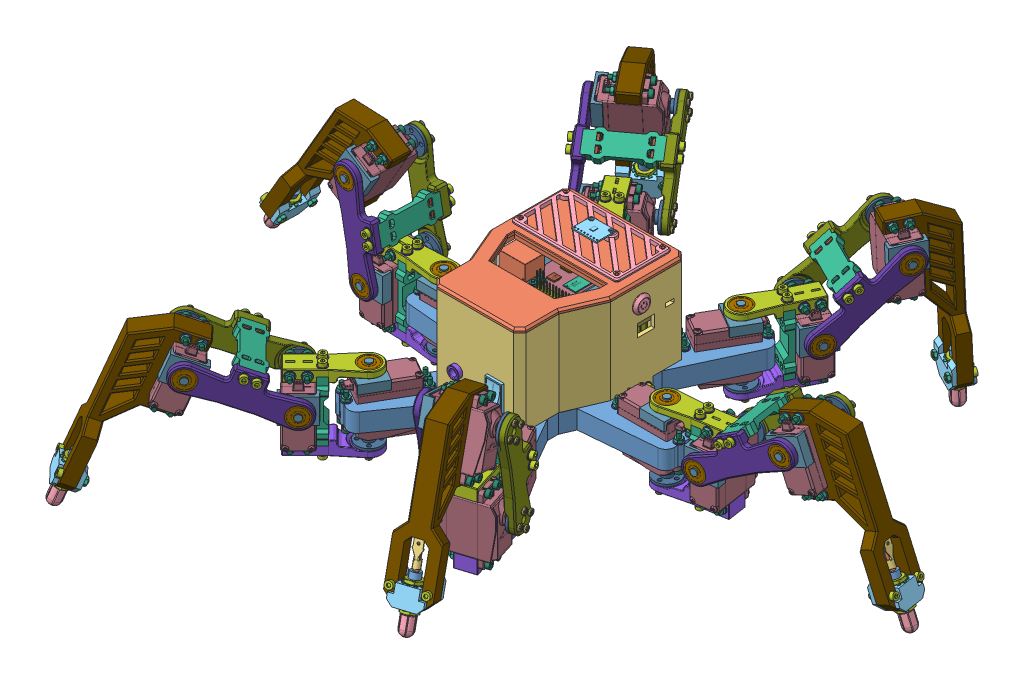
SolidWorks assembly HEXUMI_DSSERVO, configuration Default. Lengths in mm. (continued)
Components (placement in the parent): (continued)
- LEG_L-2: LEG_L [Default] at (-76.6324 -8.25 141.7647) x (0.700512 0 0.713641) z (0.713641 0 -0.700512) size (67.5 173.11 232.67) (flexible) (continued)
  - M3_SERVO_HORN_BOLT-12: M3_SERVO_HORN_BOLT [Default] at (-34.5 -12.4934 -16.7216) x (0 0.672311 -0.740269) z (0 -0.740269 -0.672311) size (4.8 7 4.8)
  - M3_SERVO_HORN_BOLT-13: M3_SERVO_HORN_BOLT [Default] at (-29.5 -35.3838 -75.416) x (0 0.520293 -0.853988) z (0 -0.853988 -0.520293) size (4.8 7 4.8)
  - M3_SERVO_HORN_BOLT-14: M3_SERVO_HORN_BOLT [Default] at (-29.5 -9.95 -10.2) x (0 0.520293 -0.853988) z (0 -0.853988 -0.520293) size (4.8 7 4.8)
  - M3_STEEL_HEX_BOLT_16MM-6: M3_STEEL_HEX_BOLT_16MM [Default] at (-36 -37.6293 -41.2662) x (0 -0.255744 -0.966745) z (0 -0.966745 0.255744) size (5.68 19 5.68)
  - M3_STEEL_HEX_BOLT_16MM-7: M3_STEEL_HEX_BOLT_16MM [Default] at (31.5 -37.6293 -41.2662) x (0 0.850981 0.525196) z (0 -0.525196 0.850981) size (5.68 19 5.68)
  - M3_STEEL_HEX_BOLT_16MM-8: M3_STEEL_HEX_BOLT_16MM [Default] at (-36 -34.7226 -33.8129) x (0 -0.563912 -0.825835) z (0 -0.825835 0.563912) size (5.68 19 5.68)
  - M3_WASHER-10: M3_WASHER [Default] at (28.5 -37.6293 -41.2662) x (0 0.320127 0.947375) z (0 -0.947375 0.320127) size (7 0.5 7)
  - M3_WASHER-11: M3_WASHER [Default] at (-32.5 -37.6293 -41.2662) x (0 0.222061 0.975033) z (0 -0.975033 0.222061) size (7 0.5 7)
  - M3_WASHER-12: M3_WASHER [Default] at (-32.5 -34.7226 -33.8129) x (0 0.409501 0.91231) z (0 -0.91231 0.409501) size (7 0.5 7)
  - M3_SQUARE_NUT-10: M3_SQUARE_NUT [Default] at (14.7 -37.6293 -41.2662) x (0 0.36334 0.931657) z (0 -0.931657 0.36334) size (5.3 1.7 5.3)
  - M3_SQUARE_NUT-11: M3_SQUARE_NUT [Default] at (14.7 -34.7226 -33.8129) x (0 0.36334 0.931657) z (0 -0.931657 0.36334) size (5.3 1.7 5.3)
  - M3_SQUARE_NUT-12: M3_SQUARE_NUT [Default] at (-17.5 -37.6293 -41.2662) x (0 0.36334 0.931657) z (0 -0.931657 0.36334) size (5.3 1.7 5.3)
  - SERVO_ASM-3: SERVO_ASM [Default] at (-25.8 -35.3838 -75.416) x (0 0.932062 -0.3623) z (-1 0 0) size (87.25 24.4 54.8)
    - SW2020 DS3225MG Servo 25Kg 4.8-6.8V-2: SW2020 DS3225MG Servo 25Kg 4.8-6.8V [Default] at origin size (54.3 20.4 45.91)
    - SERVO_CLIP-1: SERVO_CLIP [Default] at (0 0 -45.6) x (-1 0 0) z (0 0 -1) size (20 24.4 14.2)
  - M3_STEEL_HEX_BOLT-6: M3_STEEL_HEX_BOLT [Default] at (-14.2 -47.3668 -65.3936) x (0 -0.933228 -0.359286) z (0 -0.359286 0.933228) size (5.68 28 5.68)
  - M3_STEEL_HEX_BOLT-7: M3_STEEL_HEX_BOLT [Default] at (-14.2 -1.1366 -83.3637) x (0 -0.933228 -0.359286) z (0 -0.359286 0.933228) size (5.68 28 5.68)
  - M3_STEEL_HEX_BOLT-8: M3_STEEL_HEX_BOLT [Default] at (-14.2 -4.7596 -92.6843) x (0 -0.933228 -0.359286) z (0 -0.359286 0.933228) size (5.68 28 5.68)
  - M3_WASHER-13: M3_WASHER [Default] at (8.5 -50.9898 -74.7142) x (0 -0.744989 0.667077) z (0 -0.667077 -0.744989) size (7 0.5 7)
  - M3_WASHER-14: M3_WASHER [Default] at (8.5 -1.1366 -83.3637) x (0 0.510645 0.859791) z (0 -0.859791 0.510645) size (7 0.5 7)
  - M3_WASHER-15: M3_WASHER [Default] at (8.5 -47.3668 -65.3936) x (0 -0.855136 -0.518404) z (0 0.518404 -0.855136) size (7 0.5 7)
  - M3_HEX_NUT-9: M3_HEX_NUT [Default] at (8.5 -50.9898 -74.7142) x (0 -0.742673 0.669654) z (0 0.669654 0.742673) size (6.98 2.4 5.5)
  - M3_HEX_NUT-10: M3_HEX_NUT [Default] at (8.5 -47.3668 -65.3936) x (0 -0.972142 0.234393) z (0 0.234393 0.972142) size (6.98 2.4 5.5)
  - M3_HEX_NUT-11: M3_HEX_NUT [Default] at (8.5 -4.7596 -92.6843) x (0 -0.862059 0.506808) z (0 0.506808 0.862059) size (6.98 2.4 5.5)
  - M3_WASHER-17: M3_WASHER [Default] at (8.5 -4.7596 -92.6843) x (0 -0.944852 -0.327497) z (0 0.327497 -0.944852) size (7 0.5 7)
  - M3_SERVO_HORN_BOLT-15: M3_SERVO_HORN_BOLT [Default] at (0 28.25 30) x (0.299137 0 -0.95421) z (-0.95421 0 -0.299137) size (4.8 7 4.8)
  - TIBIA_V2_ASM-1: TIBIA_V2_ASM [Default] at (0 -35.2725 -75.4056) x (-1 0 0) z (0 -0.932062 0.3623) size (32.11 50.6 145.7)
    - TIBIA_V2-1: TIBIA_V2 [Default] at origin size (32 47.6 127.94)
    - LIMIT_SWITCH-1: LIMIT_SWITCH [Default] at (0 32.3524 -111.7407) x (-0.992713 0.1205 0) z (0.1205 0.992713 0) size (13.8 62.3 13.8) (flexible)
      - LIMIT_SWITCH_SLEEVE-1: LIMIT_SWITCH_SLEEVE [Default] at origin size (7.7 25.25 7.7)
      - LIMIT_SWITCH_SHAFT-1: LIMIT_SWITCH_SHAFT [Default] at (0 5.5422 0) x (-0.210419 0 -0.977611) z (0.977611 0 -0.210419) size (5 52 5)
      - LIMIT_SWITCH_LIMITER-1: LIMIT_SWITCH_LIMITER [Default] at (0 26.0422 0) x (-0.600712 0 -0.799465) z (0.799465 0 -0.600712) size (6.64 21.41 7.08)
      - RUBBER_CAP-1: RUBBER_CAP [Default] at (0 -9.9578 0) x (0.575853 0 -0.817553) z (0.817553 0 0.575853) size (10 14 10)
    - FOOT_HOLD-1: FOOT_HOLD [Default] at (0 32.3524 -108.9407) x (1 0 0) z (0 -1 0) size (32 22 16)
    - LIMIT_SWITCH_WASHER-1: LIMIT_SWITCH_WASHER [Default] at (0 32.3524 -93.5407) x (0.999093 -0.042592 0) z (0.042592 0.999093 0) size (14.82 0.4 15)
    - LIMIT_SWITCH_WASHER-2: LIMIT_SWITCH_WASHER [Default] at (0 32.3524 -108.9407) x (0.999093 -0.042592 0) z (0.042592 0.999093 0) size (14.82 0.4 15)
    - LIMIT_SWITCH_NUT-1: LIMIT_SWITCH_NUT [Default] at (0 32.3524 -92.3407) x (0.997292 -0.073548 0) z (0.073548 0.997292 0) size (13.86 2.4 12)
    - LIMIT_SWITCH_NUT-2: LIMIT_SWITCH_NUT [Default] at (0 32.3524 -110.5407) x (0.999648 -0.026514 0) z (0.026514 0.999648 0) size (13.86 2.4 12)
    - M3_HEX_NUT-1: M3_HEX_NUT [Default] at (-12 21.9524 -96.9407) x (-0.996596 0 -0.082443) z (0.082443 0 -0.996596) size (6.98 2.4 5.5)
    - M3_HEX_NUT-2: M3_HEX_NUT [Default] at (12 21.9524 -96.9407) x (-0.491735 0 -0.870745) z (0.870745 0 -0.491735) size (6.98 2.4 5.5)
    - M3_STEEL_HEX_BOLT_16MM-1: M3_STEEL_HEX_BOLT_16MM [Default] at (-12 40.3524 -96.9407) x (-0.809803 0 -0.586702) z (-0.586702 0 0.809803) size (5.68 19 5.68)
    - M3_STEEL_HEX_BOLT_16MM-2: M3_STEEL_HEX_BOLT_16MM [Default] at (12 40.3524 -96.9407) x (-0.933551 0 -0.358443) z (-0.358443 0 0.933551) size (5.68 19 5.68)
- LEG_L-3: LEG_L [Default] at (-120.0853 -8.25 24.3604) x (-0.031319 0 0.999509) z (0.999509 0 0.031319) size (67.5 177.61 179.91) (flexible)
  - LINK-1: LINK [Default] at origin size (20 48.5 7)
  - COXA_BEARING-1: COXA_BEARING [Default] at (0 -29.25 30) size (20 9.2 60)
  - COXA_SERVO-1: COXA_SERVO [Default] at (0 31.25 30) x (-1 0 0) z (0 0 1) size (20 11.2 60)
  - BEARING-1: BEARING [Default] at (0 -24.25 30) x (-0.081882 0 0.996642) z (0 -1 0) size (16 16 5)
  - HORN-1: HORN [Default] at (0 26.25 30) x (0 0 -1) z (0 -1 0) size (20 20 4.6)
  - M3_SQUARE_NUT-1: M3_SQUARE_NUT [Default] at (-4 16.25 3.5) x (0.988939 0 -0.14832) z (0.14832 0 0.988939) size (5.3 1.7 5.3)
  - M3_STEEL_HEX_BOLT_16MM-1: M3_STEEL_HEX_BOLT_16MM [Default] at (4 34.75 3.5) x (-0.949613 0 0.313425) z (0.313425 0 0.949613) size (5.68 19 5.68)
  - M3_WASHER-1: M3_WASHER [Default] at (4 31.25 3.5) x (0.934731 0 0.355356) z (-0.355356 0 0.934731) size (7 0.5 7)
  - M3_SERVO_HORN_BOLT-1: M3_SERVO_HORN_BOLT [Default] at (-7 33.25 30) x (-0.685901 0 -0.727695) z (-0.727695 0 0.685901) size (4.8 7 4.8)
  - M3_SERVO_HORN_BOLT-2: M3_SERVO_HORN_BOLT [Default] at (7 33.25 30) x (-0.685901 0 -0.727695) z (-0.727695 0 0.685901) size (4.8 7 4.8)
  - M3_SERVO_HORN_BOLT-3: M3_SERVO_HORN_BOLT [Default] at (0 33.25 37) x (-0.685901 0 -0.727695) z (-0.727695 0 0.685901) size (4.8 7 4.8)
  - M3_SERVO_HORN_BOLT-4: M3_SERVO_HORN_BOLT [Default] at (0 33.25 23) x (-0.685901 0 -0.727695) z (-0.727695 0 0.685901) size (4.8 7 4.8)
  - M3_SQUARE_NUT-2: M3_SQUARE_NUT [Default] at (4 16.25 3.5) x (0.988939 0 -0.14832) z (0.14832 0 0.988939) size (5.3 1.7 5.3)
  - M3_SQUARE_NUT-3: M3_SQUARE_NUT [Default] at (-4 -15.95 3.5) x (0.988939 0 -0.14832) z (0.14832 0 0.988939) size (5.3 1.7 5.3)
  - M3_SQUARE_NUT-4: M3_SQUARE_NUT [Default] at (4 -15.95 3.5) x (0.988939 0 -0.14832) z (0.14832 0 0.988939) size (5.3 1.7 5.3)
  - M3_STEEL_HEX_BOLT_16MM-2: M3_STEEL_HEX_BOLT_16MM [Default] at (-4 -32.75 3.5) x (0.988939 0 -0.14832) z (0.14832 0 0.988939) size (5.68 19 5.68)
  - M3_STEEL_HEX_BOLT_16MM-3: M3_STEEL_HEX_BOLT_16MM [Default] at (4 -32.75 3.5) x (0.988939 0 -0.14832) z (0.14832 0 0.988939) size (5.68 19 5.68)
  - M3_STEEL_HEX_BOLT_16MM-4: M3_STEEL_HEX_BOLT_16MM [Default] at (-4 34.75 3.5) x (-0.85786 0 0.513883) z (0.513883 0 0.85786) size (5.68 19 5.68)
  - M3_WASHER-2: M3_WASHER [Default] at (4 -29.75 3.5) x (0.985952 0 -0.167027) z (0.167027 0 0.985952) size (7 0.5 7)
  - M3_WASHER-3: M3_WASHER [Default] at (-4 -29.75 3.5) x (0.922631 0 -0.385683) z (0.385683 0 0.922631) size (7 0.5 7)
  - M3_WASHER-4: M3_WASHER [Default] at (-4 31.25 3.5) x (0.993655 0 0.112474) z (-0.112474 0 0.993655) size (7 0.5 7)
  - SERVO_ASM-1: SERVO_ASM [Default] at (-25.8 -9.95 -10.2) x (0 1 0) z (-1 0 0) size (87.25 24.4 54.8)
    - SW2020 DS3225MG Servo 25Kg 4.8-6.8V-2: SW2020 DS3225MG Servo 25Kg 4.8-6.8V [Default] at origin size (54.3 20.4 45.91)
    - SERVO_CLIP-1: SERVO_CLIP [Default] at (0 0 -45.6) x (-1 0 0) z (0 0 -1) size (20 24.4 14.2)
  - SERVO_ASM-2: SERVO_ASM [Default] at (0 24.55 30) x (-0.031319 0 0.999509) z (0 1 0) size (87.25 24.4 54.8)
    - SW2020 DS3225MG Servo 25Kg 4.8-6.8V-2: SW2020 DS3225MG Servo 25Kg 4.8-6.8V [Default] at origin size (54.3 20.4 45.91)
    - SERVO_CLIP-1: SERVO_CLIP [Default] at (0 0 -45.6) x (-1 0 0) z (0 0 -1) size (20 24.4 14.2)
  - M3_HEX_NUT-1: M3_HEX_NUT [Default] at (10.4 -24.75 -15.2) x (0 0.554401 -0.83225) z (0 0.83225 0.554401) size (6.98 2.4 5.5)
  - M3_SQUARE_NUT-5: M3_SQUARE_NUT [Default] at (0.85 24.85 -15.2) x (0 0 -1) z (0 1 0) size (5.3 1.7 5.3)
  - M3_STEEL_HEX_BOLT-1: M3_STEEL_HEX_BOLT [Default] at (-14.2 -24.75 -5.2) x (0 -0.390994 0.920393) z (0 0.920393 0.390994) size (5.68 28 5.68)
  - M3_WASHER-5: M3_WASHER [Default] at (8 -24.75 -5.2) x (0 -0.313666 0.949533) z (0 0.949533 0.313666) size (7 0.5 7)
  - M3_WASHER-6: M3_WASHER [Default] at (8 -24.75 -15.2) x (0 -0.313666 0.949533) z (0 0.949533 0.313666) size (7 0.5 7)
  - M3_WASHER-7: M3_WASHER [Default] at (8 24.85 -15.2) x (0 -0.313666 0.949533) z (0 0.949533 0.313666) size (7 0.5 7)
  - M3_WASHER-8: M3_WASHER [Default] at (8 24.85 -5.2) x (0 -0.313666 0.949533) z (0 0.949533 0.313666) size (7 0.5 7)
  - M3_STEEL_HEX_BOLT-2: M3_STEEL_HEX_BOLT [Default] at (-14.2 24.85 -15.2) x (0 -0.835258 0.549858) z (0 0.549858 0.835258) size (5.68 28 5.68)
  - M3_STEEL_HEX_BOLT-3: M3_STEEL_HEX_BOLT [Default] at (-14.2 -24.75 -15.2) x (0 0.230066 0.973175) z (0 0.973175 -0.230066) size (5.68 28 5.68)
  - M3_STEEL_HEX_BOLT-4: M3_STEEL_HEX_BOLT [Default] at (-14.2 24.85 -5.2) x (0 -0.984641 0.17459) z (0 0.17459 0.984641) size (5.68 28 5.68)
  - M3_SQUARE_NUT-6: M3_SQUARE_NUT [Default] at (0.85 -24.75 -5.2) x (0 1 0) z (0 0 1) size (5.3 1.7 5.3)
  - M3_SQUARE_NUT-7: M3_SQUARE_NUT [Default] at (0.85 -24.75 -15.2) x (0 1 0) z (0 0 1) size (5.3 1.7 5.3)
  - M3_SQUARE_NUT-8: M3_SQUARE_NUT [Default] at (0.85 24.85 -5.2) x (0 0 -1) z (0 1 0) size (5.3 1.7 5.3)
  - M3_HEX_NUT-2: M3_HEX_NUT [Default] at (10.4 -24.75 -5.2) x (0 0.450627 -0.892712) z (0 0.892712 0.450627) size (6.98 2.4 5.5)
  - M3_HEX_NUT-3: M3_HEX_NUT [Default] at (10.9 24.85 -5.2) x (0 0.387589 -0.921832) z (0 0.921832 0.387589) size (6.98 2.4 5.5)
  - M3_HEX_NUT-4: M3_HEX_NUT [Default] at (10.9 24.85 -15.2) x (0 0.281781 -0.959479) z (0 0.959479 0.281781) size (6.98 2.4 5.5)
  - FEMUR_SERVO-1: FEMUR_SERVO [Default] at (-32.5 -78.7023 -23.3578) x (1 0 0) z (0 -0.982175 -0.187968) size (10 28 90)
  - FEMUR_BEARING-1: FEMUR_BEARING [Default] at (28 -9.95 -10.2) x (-1 0 0) z (0 0.982175 0.187968) size (8 28 90)
  - LINK-2: LINK [Default] at (-1.25 -47.7096 0.9003) x (0 -0.982175 -0.187968) z (0 0.187968 -0.982175) size (20 48.5 7)
  - BEARING-2: BEARING [Default] at (28 -9.95 -10.2) x (0 0.418384 0.90827) z (-1 0 0) size (16 16 5)
  - HORN-2: HORN [Default] at (-27.5 -9.95 -10.2) x (0 -0.187968 0.982175) z (1 0 0) size (20 20 4.6)
  - BEARING-3: BEARING [Default] at (28 -78.7023 -23.3578) x (0 0.417885 0.9085) z (-1 0 0) size (16 16 5)
  - HORN-3: HORN [Default] at (-27.5 -78.7023 -23.3578) x (0 0.982175 0.187968) z (1 0 0) size (20 20 4.6)
  - M3_HEX_NUT-5: M3_HEX_NUT [Default] at (8.5 -46.1809 -36.7145) x (0 -0.996607 0.082307) z (0 0.082307 0.996607) size (6.98 2.4 5.5)
  - M3_SERVO_HORN_BOLT-5: M3_SERVO_HORN_BOLT [Default] at (-34.5 -11.2658 -3.3248) x (0 0.998165 -0.060547) z (0 -0.060547 -0.998165) size (4.8 7 4.8)
  - M3_SQUARE_NUT-9: M3_SQUARE_NUT [Default] at (-17.5 -43.123 -1.7855) x (0 0.982175 0.187968) z (0 -0.187968 0.982175) size (5.3 1.7 5.3)
  - M3_STEEL_HEX_BOLT-5: M3_STEEL_HEX_BOLT [Default] at (-14.2 -93.9918 -20.1531) x (0 -0.933228 -0.359286) z (0 -0.359286 0.933228) size (5.68 28 5.68)
  - M3_STEEL_HEX_BOLT_16MM-5: M3_STEEL_HEX_BOLT_16MM [Default] at (31.5 -43.123 -1.7855) x (0 0.963892 0.266294) z (0 -0.266294 0.963892) size (5.68 19 5.68)
  - M3_WASHER-9: M3_WASHER [Default] at (28.5 -43.123 -1.7855) x (0 0.36047 0.932771) z (0 -0.932771 0.36047) size (7 0.5 7)
  - M3_SERVO_HORN_BOLT-6: M3_SERVO_HORN_BOLT [Default] at (-34.5 -8.6342 -17.0752) x (0 0.373361 -0.927686) z (0 -0.927686 -0.373361) size (4.8 7 4.8)
  - M3_SERVO_HORN_BOLT-7: M3_SERVO_HORN_BOLT [Default] at (-34.5 -71.827 -22.042) x (0 0.325507 -0.94554) z (0 -0.94554 -0.325507) size (4.8 7 4.8)
  - M3_SERVO_HORN_BOLT-8: M3_SERVO_HORN_BOLT [Default] at (-34.5 -77.3865 -30.233) x (0 0.184546 -0.982824) z (0 -0.982824 -0.184546) size (4.8 7 4.8)
  - M3_SERVO_HORN_BOLT-9: M3_SERVO_HORN_BOLT [Default] at (-34.5 -80.018 -16.4825) x (0 0.681327 -0.731979) z (0 -0.731979 -0.681327) size (4.8 7 4.8)
  - M3_SERVO_HORN_BOLT-10: M3_SERVO_HORN_BOLT [Default] at (-34.5 -85.5775 -24.6735) x (0 0.520293 -0.853988) z (0 -0.853988 -0.520293) size (4.8 7 4.8)
  - M3_SERVO_HORN_BOLT-11: M3_SERVO_HORN_BOLT [Default] at (-34.5 -3.0748 -8.8842) x (0 -0.171182 -0.985239) z (0 -0.985239 0.171182) size (4.8 7 4.8)
  - M3_SERVO_HORN_BOLT-12: M3_SERVO_HORN_BOLT [Default] at (-34.5 -16.8252 -11.5158) x (0 0.672311 -0.740269) z (0 -0.740269 -0.672311) size (4.8 7 4.8)
  - M3_SERVO_HORN_BOLT-13: M3_SERVO_HORN_BOLT [Default] at (-29.5 -78.7023 -23.3578) x (0 0.520293 -0.853988) z (0 -0.853988 -0.520293) size (4.8 7 4.8)
  - M3_SERVO_HORN_BOLT-14: M3_SERVO_HORN_BOLT [Default] at (-29.5 -9.95 -10.2) x (0 0.520293 -0.853988) z (0 -0.853988 -0.520293) size (4.8 7 4.8)
  - M3_STEEL_HEX_BOLT_16MM-6: M3_STEEL_HEX_BOLT_16MM [Default] at (-36 -50.9804 -3.2892) x (0 -0.255744 -0.966745) z (0 -0.966745 0.255744) size (5.68 19 5.68)
  - M3_STEEL_HEX_BOLT_16MM-7: M3_STEEL_HEX_BOLT_16MM [Default] at (31.5 -50.9804 -3.2892) x (0 0.850981 0.525196) z (0 -0.525196 0.850981) size (5.68 19 5.68)
  - M3_STEEL_HEX_BOLT_16MM-8: M3_STEEL_HEX_BOLT_16MM [Default] at (-36 -43.123 -1.7855) x (0 -0.563912 -0.825835) z (0 -0.825835 0.563912) size (5.68 19 5.68)
  - M3_WASHER-10: M3_WASHER [Default] at (28.5 -50.9804 -3.2892) x (0 0.320127 0.947375) z (0 -0.947375 0.320127) size (7 0.5 7)
  - M3_WASHER-11: M3_WASHER [Default] at (-32.5 -50.9804 -3.2892) x (0 0.222061 0.975033) z (0 -0.975033 0.222061) size (7 0.5 7)
  - M3_WASHER-12: M3_WASHER [Default] at (-32.5 -43.123 -1.7855) x (0 0.409501 0.91231) z (0 -0.91231 0.409501) size (7 0.5 7)
  - M3_SQUARE_NUT-10: M3_SQUARE_NUT [Default] at (14.7 -50.9804 -3.2892) x (0 0.982175 0.187968) z (0 -0.187968 0.982175) size (5.3 1.7 5.3)
  - M3_SQUARE_NUT-11: M3_SQUARE_NUT [Default] at (14.7 -43.123 -1.7855) x (0 0.982175 0.187968) z (0 -0.187968 0.982175) size (5.3 1.7 5.3)
  - M3_SQUARE_NUT-12: M3_SQUARE_NUT [Default] at (-17.5 -50.9804 -3.2892) x (0 0.982175 0.187968) z (0 -0.187968 0.982175) size (5.3 1.7 5.3)
  - SERVO_ASM-3: SERVO_ASM [Default] at (-25.8 -78.7023 -23.3578) x (0 0.861589 -0.507606) z (-1 0 0) size (87.25 24.4 54.8)
    - SW2020 DS3225MG Servo 25Kg 4.8-6.8V-2: SW2020 DS3225MG Servo 25Kg 4.8-6.8V [Default] at origin size (54.3 20.4 45.91)
    - SERVO_CLIP-1: SERVO_CLIP [Default] at (0 0 -45.6) x (-1 0 0) z (0 0 -1) size (20 24.4 14.2)
  - M3_STEEL_HEX_BOLT-6: M3_STEEL_HEX_BOLT [Default] at (-14.2 -88.9158 -11.5372) x (0 -0.933228 -0.359286) z (0 -0.359286 0.933228) size (5.68 28 5.68)
  - M3_STEEL_HEX_BOLT-7: M3_STEEL_HEX_BOLT [Default] at (-14.2 -46.1809 -36.7145) x (0 -0.933228 -0.359286) z (0 -0.359286 0.933228) size (5.68 28 5.68)
  - M3_STEEL_HEX_BOLT-8: M3_STEEL_HEX_BOLT [Default] at (-14.2 -51.257 -45.3304) x (0 -0.933228 -0.359286) z (0 -0.359286 0.933228) size (5.68 28 5.68)
  - M3_WASHER-13: M3_WASHER [Default] at (8.5 -93.9918 -20.1531) x (0 -0.744989 0.667077) z (0 -0.667077 -0.744989) size (7 0.5 7)
  - M3_WASHER-14: M3_WASHER [Default] at (8.5 -46.1809 -36.7145) x (0 0.510645 0.859791) z (0 -0.859791 0.510645) size (7 0.5 7)
  - M3_WASHER-15: M3_WASHER [Default] at (8.5 -88.9158 -11.5372) x (0 -0.855136 -0.518404) z (0 0.518404 -0.855136) size (7 0.5 7)
  - M3_HEX_NUT-9: M3_HEX_NUT [Default] at (8.5 -93.9918 -20.1531) x (0 -0.742673 0.669654) z (0 0.669654 0.742673) size (6.98 2.4 5.5)
  - M3_HEX_NUT-10: M3_HEX_NUT [Default] at (8.5 -88.9158 -11.5372) x (0 -0.972142 0.234393) z (0 0.234393 0.972142) size (6.98 2.4 5.5)
  - M3_HEX_NUT-11: M3_HEX_NUT [Default] at (8.5 -51.257 -45.3304) x (0 -0.862059 0.506808) z (0 0.506808 0.862059) size (6.98 2.4 5.5)
  - M3_WASHER-17: M3_WASHER [Default] at (8.5 -51.257 -45.3304) x (0 -0.944852 -0.327497) z (0 0.327497 -0.944852) size (7 0.5 7)
  - M3_SERVO_HORN_BOLT-15: M3_SERVO_HORN_BOLT [Default] at (0 28.25 30) x (0.063985 0 -0.997951) z (-0.997951 0 -0.063985) size (4.8 7 4.8)
  - TIBIA_V2_ASM-1: TIBIA_V2_ASM [Default] at (0 -78.5907 -23.3654) x (-1 0 0) z (0 -0.861589 0.507606) size (32.11 50.6 145.7)
    - TIBIA_V2-1: TIBIA_V2 [Default] at origin size (32 47.6 127.94)
    - LIMIT_SWITCH-1: LIMIT_SWITCH [Default] at (0 32.3524 -111.7407) x (-0.992713 0.1205 0) z (0.1205 0.992713 0) size (13.8 62.3 13.8) (flexible)
      - LIMIT_SWITCH_SLEEVE-1: LIMIT_SWITCH_SLEEVE [Default] at origin size (7.7 25.25 7.7)
      - LIMIT_SWITCH_SHAFT-1: LIMIT_SWITCH_SHAFT [Default] at (0 5.5422 0) x (-0.210419 0 -0.977611) z (0.977611 0 -0.210419) size (5 52 5)
      - LIMIT_SWITCH_LIMITER-1: LIMIT_SWITCH_LIMITER [Default] at (0 26.0422 0) x (-0.600712 0 -0.799465) z (0.799465 0 -0.600712) size (6.64 21.41 7.08)
      - RUBBER_CAP-1: RUBBER_CAP [Default] at (0 -9.9578 0) x (0.575853 0 -0.817553) z (0.817553 0 0.575853) size (10 14 10)
    - FOOT_HOLD-1: FOOT_HOLD [Default] at (0 32.3524 -108.9407) x (1 0 0) z (0 -1 0) size (32 22 16)
    - LIMIT_SWITCH_WASHER-1: LIMIT_SWITCH_WASHER [Default] at (0 32.3524 -93.5407) x (0.999093 -0.042592 0) z (0.042592 0.999093 0) size (14.82 0.4 15)
    - LIMIT_SWITCH_WASHER-2: LIMIT_SWITCH_WASHER [Default] at (0 32.3524 -108.9407) x (0.999093 -0.042592 0) z (0.042592 0.999093 0) size (14.82 0.4 15)
    - LIMIT_SWITCH_NUT-1: LIMIT_SWITCH_NUT [Default] at (0 32.3524 -92.3407) x (0.997292 -0.073548 0) z (0.073548 0.997292 0) size (13.86 2.4 12)
    - LIMIT_SWITCH_NUT-2: LIMIT_SWITCH_NUT [Default] at (0 32.3524 -110.5407) x (0.999648 -0.026514 0) z (0.026514 0.999648 0) size (13.86 2.4 12)
    - M3_HEX_NUT-1: M3_HEX_NUT [Default] at (-12 21.9524 -96.9407) x (-0.996596 0 -0.082443) z (0.082443 0 -0.996596) size (6.98 2.4 5.5)
    - M3_HEX_NUT-2: M3_HEX_NUT [Default] at (12 21.9524 -96.9407) x (-0.491735 0 -0.870745) z (0.870745 0 -0.491735) size (6.98 2.4 5.5)
    - M3_STEEL_HEX_BOLT_16MM-1: M3_STEEL_HEX_BOLT_16MM [Default] at (-12 40.3524 -96.9407) x (-0.809803 0 -0.586702) z (-0.586702 0 0.809803) size (5.68 19 5.68)
    - M3_STEEL_HEX_BOLT_16MM-2: M3_STEEL_HEX_BOLT_16MM [Default] at (12 40.3524 -96.9407) x (-0.933551 0 -0.358443) z (-0.358443 0 0.933551) size (5.68 19 5.68)
- LEG_R-1: LEG_R [Default] at (119.7539 -8.25 20.7561) x (-0.151465 0 -0.988463) z (-0.988463 0 0.151465) size (67.5 178.11 186.84) (flexible)
  - LINK-1: LINK [Default] at origin size (20 48.5 7)
  - COXA_BEARING-1: COXA_BEARING [Default] at (0 -29.25 30) size (20 9.2 60)
  - COXA_SERVO-1: COXA_SERVO [Default] at (0 31.25 30) x (-1 0 0) z (0 0 1) size (20 11.2 60)
  - BEARING-1: BEARING [Default] at (0 -24.25 30) x (0.193177 0 0.981164) z (0 -1 0) size (16 16 5)
  - HORN-1: HORN [Default] at (0 26.25 30) x (0 0 -1) z (0 -1 0) size (20 20 4.6)
  - M3_SQUARE_NUT-1: M3_SQUARE_NUT [Default] at (-4 16.25 3.5) x (0.910939 0 -0.412541) z (0.412541 0 0.910939) size (5.3 1.7 5.3)
  - M3_STEEL_HEX_BOLT_16MM-1: M3_STEEL_HEX_BOLT_16MM [Default] at (4 34.75 3.5) x (-0.828053 0 0.56065) z (0.56065 0 0.828053) size (5.68 19 5.68)
  - M3_WASHER-1: M3_WASHER [Default] at (4 31.25 3.5) x (0.996225 0 0.086813) z (-0.086813 0 0.996225) size (7 0.5 7)
  - M3_SERVO_HORN_BOLT-1: M3_SERVO_HORN_BOLT [Default] at (-7 33.25 30) x (-0.858437 0 -0.51292) z (-0.51292 0 0.858437) size (4.8 7 4.8)
  - M3_SERVO_HORN_BOLT-2: M3_SERVO_HORN_BOLT [Default] at (7 33.25 30) x (-0.858437 0 -0.51292) z (-0.51292 0 0.858437) size (4.8 7 4.8)
  - M3_SERVO_HORN_BOLT-3: M3_SERVO_HORN_BOLT [Default] at (0 33.25 37) x (-0.858437 0 -0.51292) z (-0.51292 0 0.858437) size (4.8 7 4.8)
  - M3_SERVO_HORN_BOLT-4: M3_SERVO_HORN_BOLT [Default] at (0 33.25 23) x (-0.858437 0 -0.51292) z (-0.51292 0 0.858437) size (4.8 7 4.8)
  - M3_SQUARE_NUT-2: M3_SQUARE_NUT [Default] at (4 16.25 3.5) x (0.910939 0 -0.412541) z (0.412541 0 0.910939) size (5.3 1.7 5.3)
  - M3_SQUARE_NUT-3: M3_SQUARE_NUT [Default] at (-4 -15.95 3.5) x (0.910939 0 -0.412541) z (0.412541 0 0.910939) size (5.3 1.7 5.3)
  - M3_SQUARE_NUT-4: M3_SQUARE_NUT [Default] at (4 -15.95 3.5) x (0.910939 0 -0.412541) z (0.412541 0 0.910939) size (5.3 1.7 5.3)
  - M3_STEEL_HEX_BOLT_16MM-2: M3_STEEL_HEX_BOLT_16MM [Default] at (-4 -32.75 3.5) x (0.910939 0 -0.412541) z (0.412541 0 0.910939) size (5.68 19 5.68)
  - M3_STEEL_HEX_BOLT_16MM-3: M3_STEEL_HEX_BOLT_16MM [Default] at (4 -32.75 3.5) x (0.910939 0 -0.412541) z (0.412541 0 0.910939) size (5.68 19 5.68)
  - M3_STEEL_HEX_BOLT_16MM-4: M3_STEEL_HEX_BOLT_16MM [Default] at (-4 34.75 3.5) x (-0.685084 0 0.728464) z (0.728464 0 0.685084) size (5.68 19 5.68)
  - M3_WASHER-2: M3_WASHER [Default] at (4 -29.75 3.5) x (0.902961 0 -0.429723) z (0.429723 0 0.902961) size (7 0.5 7)
  - M3_WASHER-3: M3_WASHER [Default] at (-4 -29.75 3.5) x (0.782379 0 -0.622803) z (0.622803 0 0.782379) size (7 0.5 7)
  - M3_WASHER-4: M3_WASHER [Default] at (-4 31.25 3.5) x (0.986637 0 -0.162931) z (0.162931 0 0.986637) size (7 0.5 7)
  - SERVO_ASM-1: SERVO_ASM [Default] at (25.8 -9.95 -10.2) x (0 1 0) z (1 0 0) size (87.25 24.4 54.8)
    - SW2020 DS3225MG Servo 25Kg 4.8-6.8V-2: SW2020 DS3225MG Servo 25Kg 4.8-6.8V [Default] at origin size (54.3 20.4 45.91)
    - SERVO_CLIP-1: SERVO_CLIP [Default] at (0 0 -45.6) x (-1 0 0) z (0 0 -1) size (20 24.4 14.2)
  - SERVO_ASM-2: SERVO_ASM [Default] at (0 24.55 30) x (0.151465 0 0.988463) z (0 1 0) size (87.25 24.4 54.8)
    - SW2020 DS3225MG Servo 25Kg 4.8-6.8V-2: SW2020 DS3225MG Servo 25Kg 4.8-6.8V [Default] at origin size (54.3 20.4 45.91)
    - SERVO_CLIP-1: SERVO_CLIP [Default] at (0 0 -45.6) x (-1 0 0) z (0 0 -1) size (20 24.4 14.2)
  - M3_SQUARE_NUT-5: M3_SQUARE_NUT [Default] at (0.85 24.85 -15.2) x (0 0 -1) z (0 1 0) size (5.3 1.7 5.3)
  - M3_SQUARE_NUT-6: M3_SQUARE_NUT [Default] at (0.85 -24.75 -5.2) x (0 1 0) z (0 0 1) size (5.3 1.7 5.3)
  - M3_SQUARE_NUT-7: M3_SQUARE_NUT [Default] at (0.85 -24.75 -15.2) x (0 1 0) z (0 0 1) size (5.3 1.7 5.3)
  - M3_SQUARE_NUT-8: M3_SQUARE_NUT [Default] at (0.85 24.85 -5.2) x (0 0 -1) z (0 1 0) size (5.3 1.7 5.3)
  - FEMUR_SERVO-1: FEMUR_SERVO [Default] at (32.5 -9.95 -10.2) x (-1 0 0) z (0 0.513033 0.858369) size (10 28 90)
  - FEMUR_BEARING-1: FEMUR_BEARING [Default] at (-28 -45.8623 -70.2858) x (1 0 0) z (0 -0.513033 -0.858369) size (8 28 90)
  - LINK-2: LINK [Default] at (1.25 -43.3568 -31.0083) x (0 0.513033 0.858369) z (0 0.858369 -0.513033) size (20 48.5 7)
  - BEARING-2: BEARING [Default] at (-28 -45.8623 -70.2858) x (0 0.859543 0.511064) z (1 0 0) size (16 16 5)
  - HORN-2: HORN [Default] at (27.5 -45.8623 -70.2858) x (0 -0.858369 0.513033) z (-1 0 0) size (20 20 4.6)
  - BEARING-3: BEARING [Default] at (-28 -9.95 -10.2) x (0 0.859543 0.511064) z (1 0 0) size (16 16 5)
  - HORN-3: HORN [Default] at (27.5 -9.95 -10.2) x (0 -0.513033 -0.858369) z (-1 0 0) size (20 20 4.6)
  - M3_HEX_NUT-5: M3_HEX_NUT [Default] at (-8.5 -15.0754 -86.8486) x (0 -0.795634 0.605778) z (0 -0.605778 -0.795634) size (6.98 2.4 5.5)
  - M3_SERVO_HORN_BOLT-5: M3_SERVO_HORN_BOLT [Default] at (34.5 -51.8709 -66.6946) x (0 -0.164589 0.986362) z (0 -0.986362 -0.164589) size (4.8 7 4.8)
  - M3_SQUARE_NUT-9: M3_SQUARE_NUT [Default] at (17.5 -42.4046 -36.2374) x (0 -0.513033 -0.858369) z (0 -0.858369 0.513033) size (5.3 1.7 5.3)
  - M3_STEEL_HEX_BOLT-5: M3_STEEL_HEX_BOLT [Default] at (14.2 -58.2379 -60.4448) x (0 -0.45302 0.8915) z (0 -0.8915 -0.45302) size (5.68 28 5.68)
  - M3_STEEL_HEX_BOLT_16MM-5: M3_STEEL_HEX_BOLT_16MM [Default] at (-31.5 -42.4046 -36.2374) x (0 0.164045 0.986453) z (0 0.986453 -0.164045) size (5.68 19 5.68)
  - M3_WASHER-9: M3_WASHER [Default] at (-28.5 -42.4046 -36.2374) x (0 0.889965 0.456029) z (0 0.456029 -0.889965) size (7 0.5 7)
  - M3_SERVO_HORN_BOLT-6: M3_SERVO_HORN_BOLT [Default] at (34.5 -39.8537 -73.877) x (0 -0.961641 0.27431) z (0 -0.27431 -0.961641) size (4.8 7 4.8)
  - M3_SERVO_HORN_BOLT-7: M3_SERVO_HORN_BOLT [Default] at (34.5 -13.5412 -16.2086) x (0 -0.974393 0.224852) z (0 -0.224852 -0.974393) size (4.8 7 4.8)
  - M3_SERVO_HORN_BOLT-8: M3_SERVO_HORN_BOLT [Default] at (34.5 -3.9414 -13.7912) x (0 -0.996733 0.080764) z (0 -0.080764 -0.996733) size (4.8 7 4.8)
  - M3_SERVO_HORN_BOLT-9: M3_SERVO_HORN_BOLT [Default] at (34.5 -15.9586 -6.6088) x (0 -0.79921 0.601052) z (0 -0.601052 -0.79921) size (4.8 7 4.8)
  - M3_SERVO_HORN_BOLT-10: M3_SERVO_HORN_BOLT [Default] at (34.5 -6.3588 -4.1914) x (0 -0.903711 0.428143) z (0 -0.428143 -0.903711) size (4.8 7 4.8)
  - M3_SERVO_HORN_BOLT-11: M3_SERVO_HORN_BOLT [Default] at (34.5 -49.4536 -76.2944) x (0 -0.961939 -0.273266) z (0 0.273266 -0.961939) size (4.8 7 4.8)
  - M3_SERVO_HORN_BOLT-12: M3_SERVO_HORN_BOLT [Default] at (34.5 -42.2711 -64.2772) x (0 -0.806511 0.591219) z (0 -0.591219 -0.806511) size (4.8 7 4.8)
  - M3_SERVO_HORN_BOLT-13: M3_SERVO_HORN_BOLT [Default] at (29.5 -9.95 -10.2) x (0 -0.903711 0.428143) z (0 -0.428143 -0.903711) size (4.8 7 4.8)
  - M3_SERVO_HORN_BOLT-14: M3_SERVO_HORN_BOLT [Default] at (29.5 -45.8623 -70.2858) x (0 -0.903711 0.428143) z (0 -0.428143 -0.903711) size (4.8 7 4.8)
  - M3_STEEL_HEX_BOLT_16MM-6: M3_STEEL_HEX_BOLT_16MM [Default] at (36 -38.3004 -29.3705) x (0 -0.934703 -0.35543) z (0 0.35543 -0.934703) size (5.68 19 5.68)
  - M3_STEEL_HEX_BOLT_16MM-7: M3_STEEL_HEX_BOLT_16MM [Default] at (-31.5 -38.3004 -29.3705) x (0 0.433334 0.901233) z (0 0.901233 -0.433334) size (5.68 19 5.68)
  - M3_STEEL_HEX_BOLT_16MM-8: M3_STEEL_HEX_BOLT_16MM [Default] at (36 -42.4046 -36.2374) x (0 -0.762342 -0.647175) z (0 0.647175 -0.762342) size (5.68 19 5.68)
  - M3_WASHER-10: M3_WASHER [Default] at (-28.5 -38.3004 -29.3705) x (0 0.908707 0.417435) z (0 0.417435 -0.908707) size (7 0.5 7)
  - M3_WASHER-11: M3_WASHER [Default] at (32.5 -38.3004 -29.3705) x (0 0.946468 0.322799) z (0 0.322799 -0.946468) size (7 0.5 7)
  - M3_WASHER-12: M3_WASHER [Default] at (32.5 -42.4046 -36.2374) x (0 0.864489 0.502652) z (0 0.502652 -0.864489) size (7 0.5 7)
  - M3_SQUARE_NUT-10: M3_SQUARE_NUT [Default] at (-14.7 -38.3004 -29.3705) x (0 -0.513033 -0.858369) z (0 -0.858369 0.513033) size (5.3 1.7 5.3)
  - M3_SQUARE_NUT-11: M3_SQUARE_NUT [Default] at (-14.7 -42.4046 -36.2374) x (0 -0.513033 -0.858369) z (0 -0.858369 0.513033) size (5.3 1.7 5.3)
  - M3_SQUARE_NUT-12: M3_SQUARE_NUT [Default] at (17.5 -38.3004 -29.3705) x (0 -0.513033 -0.858369) z (0 -0.858369 0.513033) size (5.3 1.7 5.3)
  - SERVO_ASM-3: SERVO_ASM [Default] at (25.8 -45.8623 -70.2858) x (0 0.939355 -0.342947) z (1 0 0) size (87.25 24.4 54.8)
    - SW2020 DS3225MG Servo 25Kg 4.8-6.8V-2: SW2020 DS3225MG Servo 25Kg 4.8-6.8V [Default] at origin size (54.3 20.4 45.91)
    - SERVO_CLIP-1: SERVO_CLIP [Default] at (0 0 -45.6) x (-1 0 0) z (0 0 -1) size (20 24.4 14.2)
  - M3_STEEL_HEX_BOLT-6: M3_STEEL_HEX_BOLT [Default] at (14.2 -61.6674 -69.8384) x (0 -0.45302 0.8915) z (0 -0.8915 -0.45302) size (5.68 28 5.68)
  - M3_STEEL_HEX_BOLT-7: M3_STEEL_HEX_BOLT [Default] at (14.2 -15.0754 -86.8486) x (0 -0.45302 0.8915) z (0 -0.8915 -0.45302) size (5.68 28 5.68)
  - M3_STEEL_HEX_BOLT-8: M3_STEEL_HEX_BOLT [Default] at (14.2 -11.6459 -77.455) x (0 -0.45302 0.8915) z (0 -0.8915 -0.45302) size (5.68 28 5.68)
  - M3_WASHER-13: M3_WASHER [Default] at (-8.5 -58.2379 -60.4448) x (0 -0.999996 0.002865) z (0 0.002865 0.999996) size (7 0.5 7)
  - M3_WASHER-14: M3_WASHER [Default] at (-8.5 -15.0754 -86.8486) x (0 -0.195932 -0.980617) z (0 -0.980617 0.195932) size (7 0.5 7)
  - M3_WASHER-15: M3_WASHER [Default] at (-8.5 -61.6674 -69.8384) x (0 -0.288509 0.957477) z (0 0.957477 0.288509) size (7 0.5 7)
  - M3_HEX_NUT-9: M3_HEX_NUT [Default] at (-8.5 -58.2379 -60.4448) x (0 -1 -0.0006) z (0 0.0006 -1) size (6.98 2.4 5.5)
  - M3_HEX_NUT-10: M3_HEX_NUT [Default] at (-8.5 -61.6674 -69.8384) x (0 -0.879232 0.476394) z (0 -0.476394 -0.879232) size (6.98 2.4 5.5)
  - M3_HEX_NUT-11: M3_HEX_NUT [Default] at (-8.5 -11.6459 -77.455) x (0 -0.979734 0.200301) z (0 -0.200301 -0.979734) size (6.98 2.4 5.5)
  - M3_WASHER-17: M3_WASHER [Default] at (-8.5 -11.6459 -77.455) x (0 -0.482932 0.875658) z (0 0.875658 0.482932) size (7 0.5 7)
  - M3_SERVO_HORN_BOLT-15: M3_SERVO_HORN_BOLT [Default] at (0 28.25 30) x (-0.210752 0 -0.97754) z (-0.97754 0 0.210752) size (4.8 7 4.8)
  - M3_HEX_NUT-12: M3_HEX_NUT [Default] at (-10.9 -24.75 -5.2) x (0 -0.133559 0.991041) z (0 0.991041 0.133559) size (6.98 2.4 5.5)
  - M3_STEEL_HEX_BOLT-9: M3_STEEL_HEX_BOLT [Default] at (14.2 -24.75 -5.2) x (0 -0.73374 -0.679431) z (0 0.679431 -0.73374) size (5.68 28 5.68)
  - M3_WASHER-18: M3_WASHER [Default] at (-8.5 -24.75 -5.2) x (0 -0.999705 0.024279) z (0 0.024279 0.999705) size (7 0.5 7)
  - M3_STEEL_HEX_BOLT-10: M3_STEEL_HEX_BOLT [Default] at (14.2 -24.75 -15.2) x (0 -0.740024 -0.67258) z (0 0.67258 -0.740024) size (5.68 28 5.68)
  - M3_STEEL_HEX_BOLT-11: M3_STEEL_HEX_BOLT [Default] at (14.2 24.85 -5.2) x (0 -0.741809 -0.670611) z (0 0.670611 -0.741809) size (5.68 28 5.68)
  - M3_STEEL_HEX_BOLT-12: M3_STEEL_HEX_BOLT [Default] at (14.2 24.85 -15.2) x (0 0.582747 -0.812654) z (0 0.812654 0.582747) size (5.68 28 5.68)
  - M3_HEX_NUT-13: M3_HEX_NUT [Default] at (-10.9 24.85 -15.2) x (0 0.525669 0.850689) z (0 0.850689 -0.525669) size (6.98 2.4 5.5)
  - M3_WASHER-19: M3_WASHER [Default] at (-8.5 24.85 -15.2) x (0 -0.601111 0.799166) z (0 0.799166 0.601111) size (7 0.5 7)
  - M3_HEX_NUT-14: M3_HEX_NUT [Default] at (-10.9 24.85 -5.2) x (0 -0.636716 -0.771098) z (0 -0.771098 0.636716) size (6.98 2.4 5.5)
  - M3_WASHER-20: M3_WASHER [Default] at (-8.5 24.85 -5.2) x (0 -0.786332 -0.617804) z (0 -0.617804 0.786332) size (7 0.5 7)
  - M3_HEX_NUT-15: M3_HEX_NUT [Default] at (-10.9 -24.75 -15.2) x (0 0.444007 -0.896023) z (0 -0.896023 -0.444007) size (6.98 2.4 5.5)
  - M3_WASHER-21: M3_WASHER [Default] at (-8.5 -24.75 -15.2) x (0 -0.943365 -0.331756) z (0 -0.331756 0.943365) size (7 0.5 7)
  - TIBIA_V2_ASM-1: TIBIA_V2_ASM [Default] at (0 -45.9391 -70.2046) x (-1 0 0) z (0 -0.939355 0.342947) size (32.11 50.6 145.7)
    - TIBIA_V2-1: TIBIA_V2 [Default] at origin size (32 47.6 127.94)
    - LIMIT_SWITCH-1: LIMIT_SWITCH [Default] at (0 32.3524 -111.7407) x (-0.992713 0.1205 0) z (0.1205 0.992713 0) size (13.8 62.3 13.8) (flexible)
      - LIMIT_SWITCH_SLEEVE-1: LIMIT_SWITCH_SLEEVE [Default] at origin size (7.7 25.25 7.7)
      - LIMIT_SWITCH_SHAFT-1: LIMIT_SWITCH_SHAFT [Default] at (0 5.5422 0) x (-0.210419 0 -0.977611) z (0.977611 0 -0.210419) size (5 52 5)
      - LIMIT_SWITCH_LIMITER-1: LIMIT_SWITCH_LIMITER [Default] at (0 26.0422 0) x (-0.600712 0 -0.799465) z (0.799465 0 -0.600712) size (6.64 21.41 7.08)
      - RUBBER_CAP-1: RUBBER_CAP [Default] at (0 -9.9578 0) x (0.575853 0 -0.817553) z (0.817553 0 0.575853) size (10 14 10)
    - FOOT_HOLD-1: FOOT_HOLD [Default] at (0 32.3524 -108.9407) x (1 0 0) z (0 -1 0) size (32 22 16)
    - LIMIT_SWITCH_WASHER-1: LIMIT_SWITCH_WASHER [Default] at (0 32.3524 -93.5407) x (0.999093 -0.042592 0) z (0.042592 0.999093 0) size (14.82 0.4 15)
    - LIMIT_SWITCH_WASHER-2: LIMIT_SWITCH_WASHER [Default] at (0 32.3524 -108.9407) x (0.999093 -0.042592 0) z (0.042592 0.999093 0) size (14.82 0.4 15)
    - LIMIT_SWITCH_NUT-1: LIMIT_SWITCH_NUT [Default] at (0 32.3524 -92.3407) x (0.997292 -0.073548 0) z (0.073548 0.997292 0) size (13.86 2.4 12)
    - LIMIT_SWITCH_NUT-2: LIMIT_SWITCH_NUT [Default] at (0 32.3524 -110.5407) x (0.999648 -0.026514 0) z (0.026514 0.999648 0) size (13.86 2.4 12)
    - M3_HEX_NUT-1: M3_HEX_NUT [Default] at (-12 21.9524 -96.9407) x (-0.996596 0 -0.082443) z (0.082443 0 -0.996596) size (6.98 2.4 5.5)
    - M3_HEX_NUT-2: M3_HEX_NUT [Default] at (12 21.9524 -96.9407) x (-0.491735 0 -0.870745) z (0.870745 0 -0.491735) size (6.98 2.4 5.5)
    - M3_STEEL_HEX_BOLT_16MM-1: M3_STEEL_HEX_BOLT_16MM [Default] at (-12 40.3524 -96.9407) x (-0.809803 0 -0.586702) z (-0.586702 0 0.809803) size (5.68 19 5.68)
    - M3_STEEL_HEX_BOLT_16MM-2: M3_STEEL_HEX_BOLT_16MM [Default] at (12 40.3524 -96.9407) x (-0.933551 0 -0.358443) z (-0.358443 0 0.933551) size (5.68 19 5.68)
- LEG_R-2: LEG_R [Default] at (64.2974 -8.25 149.3441) x (0.953158 0 -0.302473) z (-0.302473 0 -0.953158) size (67.5 178.11 186.84) (flexible)
  - LINK-1: LINK [Default] at origin size (20 48.5 7)
  - COXA_BEARING-1: COXA_BEARING [Default] at (0 -29.25 30) size (20 9.2 60)
  - COXA_SERVO-1: COXA_SERVO [Default] at (0 31.25 30) x (-1 0 0) z (0 0 1) size (20 11.2 60)
  - BEARING-1: BEARING [Default] at (0 -24.25 30) x (-0.173088 0 0.984906) z (0 -1 0) size (16 16 5)
  - HORN-1: HORN [Default] at (0 26.25 30) x (0 0 -1) z (0 -1 0) size (20 20 4.6)
  - M3_SQUARE_NUT-1: M3_SQUARE_NUT [Default] at (-4 16.25 3.5) x (0.998383 0 -0.056849) z (0.056849 0 0.998383) size (5.3 1.7 5.3)
  - M3_STEEL_HEX_BOLT_16MM-1: M3_STEEL_HEX_BOLT_16MM [Default] at (4 34.75 3.5) x (-0.974389 0 0.224868) z (0.224868 0 0.974389) size (5.68 19 5.68)
  - M3_WASHER-1: M3_WASHER [Default] at (4 31.25 3.5) x (0.898136 0 0.439718) z (-0.439718 0 0.898136) size (7 0.5 7)
  - M3_SERVO_HORN_BOLT-1: M3_SERVO_HORN_BOLT [Default] at (-7 33.25 30) x (-0.616155 0 -0.787625) z (-0.787625 0 0.616155) size (4.8 7 4.8)
  - M3_SERVO_HORN_BOLT-2: M3_SERVO_HORN_BOLT [Default] at (7 33.25 30) x (-0.616155 0 -0.787625) z (-0.787625 0 0.616155) size (4.8 7 4.8)
  - M3_SERVO_HORN_BOLT-3: M3_SERVO_HORN_BOLT [Default] at (0 33.25 37) x (-0.616155 0 -0.787625) z (-0.787625 0 0.616155) size (4.8 7 4.8)
  - M3_SERVO_HORN_BOLT-4: M3_SERVO_HORN_BOLT [Default] at (0 33.25 23) x (-0.616155 0 -0.787625) z (-0.787625 0 0.616155) size (4.8 7 4.8)
  - M3_SQUARE_NUT-2: M3_SQUARE_NUT [Default] at (4 16.25 3.5) x (0.998383 0 -0.056849) z (0.056849 0 0.998383) size (5.3 1.7 5.3)
  - M3_SQUARE_NUT-3: M3_SQUARE_NUT [Default] at (-4 -15.95 3.5) x (0.998383 0 -0.056849) z (0.056849 0 0.998383) size (5.3 1.7 5.3)
  - M3_SQUARE_NUT-4: M3_SQUARE_NUT [Default] at (4 -15.95 3.5) x (0.998383 0 -0.056849) z (0.056849 0 0.998383) size (5.3 1.7 5.3)
  - M3_STEEL_HEX_BOLT_16MM-2: M3_STEEL_HEX_BOLT_16MM [Default] at (-4 -32.75 3.5) x (0.998383 0 -0.056849) z (0.056849 0 0.998383) size (5.68 19 5.68)
  - M3_STEEL_HEX_BOLT_16MM-3: M3_STEEL_HEX_BOLT_16MM [Default] at (4 -32.75 3.5) x (0.998383 0 -0.056849) z (0.056849 0 0.998383) size (5.68 19 5.68)
  - M3_STEEL_HEX_BOLT_16MM-4: M3_STEEL_HEX_BOLT_16MM [Default] at (-4 34.75 3.5) x (-0.901439 0 0.432907) z (0.432907 0 0.901439) size (5.68 19 5.68)
  - M3_WASHER-2: M3_WASHER [Default] at (4 -29.75 3.5) x (0.997127 0 -0.075751) z (0.075751 0 0.997127) size (7 0.5 7)
  - M3_WASHER-3: M3_WASHER [Default] at (-4 -29.75 3.5) x (0.954159 0 -0.299299) z (0.299299 0 0.954159) size (7 0.5 7)
  - M3_WASHER-4: M3_WASHER [Default] at (-4 31.25 3.5) x (0.979122 0 0.203275) z (-0.203275 0 0.979122) size (7 0.5 7)
  - SERVO_ASM-1: SERVO_ASM [Default] at (25.8 -9.95 -10.2) x (0 1 0) z (1 0 0) size (87.25 24.4 54.8)
    - SW2020 DS3225MG Servo 25Kg 4.8-6.8V-2: SW2020 DS3225MG Servo 25Kg 4.8-6.8V [Default] at origin size (54.3 20.4 45.91)
    - SERVO_CLIP-1: SERVO_CLIP [Default] at (0 0 -45.6) x (-1 0 0) z (0 0 -1) size (20 24.4 14.2)
  - SERVO_ASM-2: SERVO_ASM [Default] at (0 24.55 30) x (-0.21463 0 0.976696) z (0 1 0) size (87.25 24.4 54.8)
    - SW2020 DS3225MG Servo 25Kg 4.8-6.8V-2: SW2020 DS3225MG Servo 25Kg 4.8-6.8V [Default] at origin size (54.3 20.4 45.91)
    - SERVO_CLIP-1: SERVO_CLIP [Default] at (0 0 -45.6) x (-1 0 0) z (0 0 -1) size (20 24.4 14.2)
  - M3_SQUARE_NUT-5: M3_SQUARE_NUT [Default] at (0.85 24.85 -15.2) x (0 0 -1) z (0 1 0) size (5.3 1.7 5.3)
  - M3_SQUARE_NUT-6: M3_SQUARE_NUT [Default] at (0.85 -24.75 -5.2) x (0 1 0) z (0 0 1) size (5.3 1.7 5.3)
  - M3_SQUARE_NUT-7: M3_SQUARE_NUT [Default] at (0.85 -24.75 -15.2) x (0 1 0) z (0 0 1) size (5.3 1.7 5.3)
  - M3_SQUARE_NUT-8: M3_SQUARE_NUT [Default] at (0.85 24.85 -5.2) x (0 0 -1) z (0 1 0) size (5.3 1.7 5.3)
  - FEMUR_SERVO-1: FEMUR_SERVO [Default] at (32.5 -9.95 -10.2) x (-1 0 0) z (0 0.985259 0.171071) size (10 28 90)
  - FEMUR_BEARING-1: FEMUR_BEARING [Default] at (-28 -78.9181 -22.175) x (1 0 0) z (0 -0.985259 -0.171071) size (8 28 90)
  - LINK-2: LINK [Default] at (1.25 -47.5133 1.5472) x (0 0.985259 0.171071) z (0 0.171071 -0.985259) size (20 48.5 7)
  - BEARING-2: BEARING [Default] at (-28 -78.9181 -22.175) x (0 0.859543 0.511064) z (1 0 0) size (16 16 5)
  - HORN-2: HORN [Default] at (27.5 -78.9181 -22.175) x (0 -0.171071 0.985259) z (-1 0 0) size (20 20 4.6)
  - BEARING-3: BEARING [Default] at (-28 -9.95 -10.2) x (0 0.859543 0.511064) z (1 0 0) size (16 16 5)
  - HORN-3: HORN [Default] at (27.5 -9.95 -10.2) x (0 -0.985259 -0.171071) z (-1 0 0) size (20 20 4.6)
  - M3_HEX_NUT-5: M3_HEX_NUT [Default] at (-8.5 -47.9503 -38.3971) x (0 -0.795634 0.605778) z (0 -0.605778 -0.795634) size (6.98 2.4 5.5)
  - M3_SERVO_HORN_BOLT-5: M3_SERVO_HORN_BOLT [Default] at (34.5 -80.1156 -15.2782) x (0 -0.164589 0.986362) z (0 -0.986362 -0.164589) size (4.8 7 4.8)
  - M3_SQUARE_NUT-9: M3_SQUARE_NUT [Default] at (17.5 -50.8556 -2.5855) x (0 -0.985259 -0.171071) z (0 -0.171071 0.985259) size (5.3 1.7 5.3)
  - M3_STEEL_HEX_BOLT-5: M3_STEEL_HEX_BOLT [Default] at (14.2 -91.4015 -12.4711) x (0 -0.45302 0.8915) z (0 -0.8915 -0.45302) size (5.68 28 5.68)
  - M3_STEEL_HEX_BOLT_16MM-5: M3_STEEL_HEX_BOLT_16MM [Default] at (-31.5 -50.8556 -2.5855) x (0 0.164045 0.986453) z (0 0.986453 -0.164045) size (5.68 19 5.68)
  - M3_WASHER-9: M3_WASHER [Default] at (-28.5 -50.8556 -2.5855) x (0 0.889965 0.456029) z (0 0.456029 -0.889965) size (7 0.5 7)
  - M3_SERVO_HORN_BOLT-6: M3_SERVO_HORN_BOLT [Default] at (34.5 -77.7206 -29.0718) x (0 -0.961641 0.27431) z (0 -0.27431 -0.961641) size (4.8 7 4.8)
  - M3_SERVO_HORN_BOLT-7: M3_SERVO_HORN_BOLT [Default] at (34.5 -16.8468 -11.3975) x (0 -0.974393 0.224852) z (0 -0.224852 -0.974393) size (4.8 7 4.8)
  - M3_SERVO_HORN_BOLT-8: M3_SERVO_HORN_BOLT [Default] at (34.5 -8.7525 -17.0968) x (0 -0.996733 0.080764) z (0 -0.080764 -0.996733) size (4.8 7 4.8)
  - M3_SERVO_HORN_BOLT-9: M3_SERVO_HORN_BOLT [Default] at (34.5 -11.1475 -3.3032) x (0 -0.79921 0.601052) z (0 -0.601052 -0.79921) size (4.8 7 4.8)
  - M3_SERVO_HORN_BOLT-10: M3_SERVO_HORN_BOLT [Default] at (34.5 -3.0532 -9.0025) x (0 -0.903711 0.428143) z (0 -0.428143 -0.903711) size (4.8 7 4.8)
  - M3_SERVO_HORN_BOLT-11: M3_SERVO_HORN_BOLT [Default] at (34.5 -85.8149 -23.3725) x (0 -0.961939 -0.273266) z (0 0.273266 -0.961939) size (4.8 7 4.8)
  - M3_SERVO_HORN_BOLT-12: M3_SERVO_HORN_BOLT [Default] at (34.5 -72.0213 -20.9775) x (0 -0.806511 0.591219) z (0 -0.591219 -0.806511) size (4.8 7 4.8)
  - M3_SERVO_HORN_BOLT-13: M3_SERVO_HORN_BOLT [Default] at (29.5 -9.95 -10.2) x (0 -0.903711 0.428143) z (0 -0.428143 -0.903711) size (4.8 7 4.8)
  - M3_SERVO_HORN_BOLT-14: M3_SERVO_HORN_BOLT [Default] at (29.5 -78.9181 -22.175) x (0 -0.903711 0.428143) z (0 -0.428143 -0.903711) size (4.8 7 4.8)
  - M3_STEEL_HEX_BOLT_16MM-6: M3_STEEL_HEX_BOLT_16MM [Default] at (36 -42.9736 -1.217) x (0 -0.934703 -0.35543) z (0 0.35543 -0.934703) size (5.68 19 5.68)
  - M3_STEEL_HEX_BOLT_16MM-7: M3_STEEL_HEX_BOLT_16MM [Default] at (-31.5 -42.9736 -1.217) x (0 0.433334 0.901233) z (0 0.901233 -0.433334) size (5.68 19 5.68)
  - M3_STEEL_HEX_BOLT_16MM-8: M3_STEEL_HEX_BOLT_16MM [Default] at (36 -50.8556 -2.5855) x (0 -0.762342 -0.647175) z (0 0.647175 -0.762342) size (5.68 19 5.68)
  - M3_WASHER-10: M3_WASHER [Default] at (-28.5 -42.9736 -1.217) x (0 0.908707 0.417435) z (0 0.417435 -0.908707) size (7 0.5 7)
